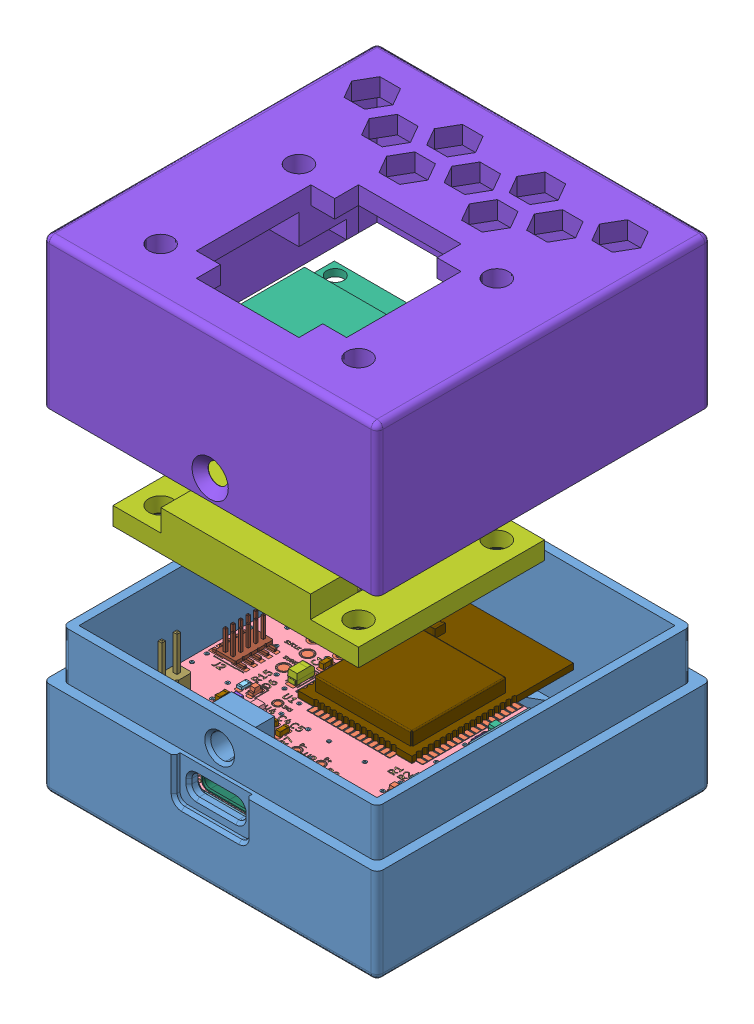
SolidWorks assembly Assem_oled, configuration Default. Lengths in mm.
Overall size (56 81 56).
54 component instances, 26 part files, 31 mates.
Components (placement in the parent):
- case-1: case [Default] at (-21.1368 5.0179 9.443) size (56 24 56)
- UWBkit_minimal-1: UWBkit_minimal [Default] at (-172.7818 2.0179 -67.157) x (1 0 0) z (0 1 0) size (49.01 48.45 15.4)
  - UWBkit_minimal.step-1: UWBkit_minimal.step [Default] at origin size (49.01 48.45 15.4)
    - LED_0603_1608Metric.step-1: LED_0603_1608Metric.step [Default] at (168.7 -85.925 1.595) x (0 -1 0) z (0 0 1) size (1.6 0.8 1.1)
    - SW_PUSH_6mm_H7.3mm.step-1: SW_PUSH_6mm_H7.3mm.step [Default] at (139.45 -64.15 1.595) x (0 -1 0) z (0 0 1) size (7.17 6 10.8)
    - SOT-23-5.step-1: SOT-23-5.step [Default] at (141 -86.775 1.595) x (-1 0 0) z (0 0 1) size (2.8 2.9 1.55)
    - R_0603_1608Metric.step-1: R_0603_1608Metric.step [Default] at (165.5 -82.3 1.595) x (0 1 0) z (0 0 1) size (1.6 0.8 0.45)
    - R_0603_1608Metric.step-2: R_0603_1608Metric.step [Default] at (135.9 -83.2 1.595) x (0 -1 0) z (0 0 1) size (1.6 0.8 0.45)
    - R_0603_1608Metric.step-3: R_0603_1608Metric.step [Default] at (163.9 -82.3 1.595) x (0 1 0) z (0 0 1) size (1.6 0.8 0.45)
    - SOT-23.step-1: SOT-23.step [Default] at (168.1 -68.7 1.595) x (0 1 0) z (0 0 1) size (2.5 3 1.2)
    - CP_EIA-3216-18_Kemet-A.step-1: CP_EIA-3216-18_Kemet-A.step [Default] at (139.6 -77.2775 1.595) x (0 -1 0) z (0 0 1) size (3.2 1.6 1.8)
    - L_0805_2012Metric.step-1: L_0805_2012Metric.step [Default] at (137.8 -86.8 1.595) x (0 1 0) z (0 0 1) size (2 1.25 1.25)
    - C_0603_1608Metric.step-1: C_0603_1608Metric.step [Default] at (139.8 -73.325 1.595) x (0 1 0) z (0 0 1) size (1.6 0.8 0.8)
    - PinSocket_1x02_P2.54mm_Vertical.step-1: PinSocket_1x02_P2.54mm_Vertical.step [Default] at (142.275 -99 1.595) x (0 -1 0) z (0 0 1) size (2.54 5.08 11.6)
    - R_0603_1608Metric.step-4: R_0603_1608Metric.step [Default] at (167.9 -65.8 1.595) x (-1 0 0) z (0 0 1) size (1.6 0.8 0.45)
    - C_0603_1608Metric.step-2: C_0603_1608Metric.step [Default] at (146 -86.8 1.595) x (0 -1 0) z (0 0 1) size (1.6 0.8 0.8)
    - PinHeader_2x05_P1.27mm_Vertical_SMD.step-1: PinHeader_2x05_P1.27mm_Vertical_SMD.step [Default] at (130.8 -78 1.595) x (-1 0 0) z (0 0 1) size (5.57 6.35 4.4)
    - R_0603_1608Metric.step-5: R_0603_1608Metric.step [Default] at (167.8 -75.7 1.595) x (0 1 0) z (0 0 1) size (1.6 0.8 0.45)
    - SOT-23.step-2: SOT-23.step [Default] at (164.5 -68.7 1.595) x (0 1 0) z (0 0 1) size (2.5 3 1.2)
    - PinHeader_1x02_P2.54mm_Vertical.step-1: PinHeader_1x02_P2.54mm_Vertical.step [Default] at (130.8 -89.325 1.595) size (2.54 5.08 11.54)
    - R_0603_1608Metric.step-6: R_0603_1608Metric.step [Default] at (164.8 -75.7 1.595) x (0 1 0) z (0 0 1) size (1.6 0.8 0.45)
    - SOT-23-3.step-1: SOT-23-3.step [Default] at (143.025 -95 1.595) x (0 -1 0) z (0 0 1) size (2.5 3 1.2)
    - PinSocket_1x04_P2.54mm_Vertical.step-1: PinSocket_1x04_P2.54mm_Vertical.step [Default] at (172.7 -79.745 1.595) x (-1 0 0) z (0 0 1) size (2.54 10.16 11.6)
    - R_0603_1608Metric.step-7: R_0603_1608Metric.step [Default] at (164.7 -65.8 1.595) size (1.6 0.8 0.45)
    - LED_0603_1608Metric.step-2: LED_0603_1608Metric.step [Default] at (163.9 -85.925 1.595) x (0 -1 0) z (0 0 1) size (1.6 0.8 1.1)
    - SOT-23.step-3: SOT-23.step [Default] at (139.025 -95 1.595) x (0 -1 0) z (0 0 1) size (2.5 3 1.2)
    - R_0603_1608Metric.step-8: R_0603_1608Metric.step [Default] at (166.3 -75.7 1.595) x (0 1 0) z (0 0 1) size (1.6 0.8 0.45)
    - SOT-23-5.step-2: SOT-23-5.step [Default] at (141.025 -90.6 1.595) x (-1 0 0) z (0 0 1) size (2.8 2.9 1.55)
    - R_0603_1608Metric.step-9: R_0603_1608Metric.step [Default] at (167.9 -64.1 1.595) size (1.6 0.8 0.45)
    - USB_C_Receptacle_GCT_USB4105-xx-A_16P_TopMnt_Horizontal.step-1: USB_C_Receptacle_GCT_USB4105-xx-A_16P_TopMnt_Horizontal.step [Default] at (151.625 -97.94 1.595) size (8.94 7.78 4.26)
    - R_0603_1608Metric.step-10: R_0603_1608Metric.step [Default] at (155.825 -90.6 1.595) x (0 1 0) z (0 0 1) size (1.6 0.8 0.45)
    - C_0603_1608Metric.step-3: C_0603_1608Metric.step [Default] at (144.1 -86.8 1.595) x (0 -1 0) z (0 0 1) size (1.6 0.8 0.8)
    - R_0603_1608Metric.step-11: R_0603_1608Metric.step [Default] at (167.11 -82.3 1.595) x (0 1 0) z (0 0 1) size (1.6 0.8 0.45)
    - C_0603_1608Metric.step-4: C_0603_1608Metric.step [Default] at (135.9 -86.8 1.595) x (0 -1 0) z (0 0 1) size (1.6 0.8 0.8)
    - LED_0603_1608Metric.step-3: LED_0603_1608Metric.step [Default] at (165.5 -85.925 1.595) x (0 -1 0) z (0 0 1) size (1.6 0.8 1.1)
    - LED_0603_1608Metric.step-4: LED_0603_1608Metric.step [Default] at (167.11 -85.925 1.595) x (0 -1 0) z (0 0 1) size (1.6 0.8 1.1)
    - SC-74-6_1.55x2.9mm_P0.95mm.step-1: SC-74-6_1.55x2.9mm_P0.95mm.step [Default] at (151.625 -90.6 1.595) x (-1 0 0) z (0 0 1) size (2.7 2.9 1.18)
    - R_0603_1608Metric.step-12: R_0603_1608Metric.step [Default] at (144.1 -90.6 1.595) x (0 1 0) z (0 0 1) size (1.6 0.8 0.45)
    - LED_0603_1608Metric.step-5: LED_0603_1608Metric.step [Default] at (137.8 -83.2 1.595) x (0 -1 0) z (0 0 1) size (1.6 0.8 1.1)
    - C_0603_1608Metric.step-5: C_0603_1608Metric.step [Default] at (158.325 -99.2 1.595) x (0 -1 0) z (0 0 1) size (1.6 0.8 0.8)
    - R_0603_1608Metric.step-13: R_0603_1608Metric.step [Default] at (164.7 -64.1 1.595) size (1.6 0.8 0.45)
    - R_0603_1608Metric.step-14: R_0603_1608Metric.step [Default] at (158.325 -96.1 1.595) x (0 1 0) z (0 0 1) size (1.6 0.8 0.45)
    - LED_RGB_Wuerth-PLCC4_3.2x2.8mm_150141M173100.step-1: LED_RGB_Wuerth-PLCC4_3.2x2.8mm_150141M173100.step [Default] at (166.3 -72.5 1.595) size (3.5 2.8 2.05)
    - DWM3001C.step-1: DWM3001C.step [Default] at (151.6 -66.71 2.595) size (19.13 27.1 3.2)
    - R_0603_1608Metric.step-15: R_0603_1608Metric.step [Default] at (168.7 -82.3 1.595) x (0 1 0) z (0 0 1) size (1.6 0.8 0.45)
    - R_0603_1608Metric.step-16: R_0603_1608Metric.step [Default] at (147.325 -90.6 1.595) x (0 1 0) z (0 0 1) size (1.6 0.8 0.45)
    - BatteryHolder_Keystone_1058_1x2032.step-1: BatteryHolder_Keystone_1058_1x2032.step [Default] at (151.625 -82.7 -0.085) x (1 0 0) z (0 0 -1) size (31.86 16 5.08)
    - UWBkit_minimal_pad.step-1: UWBkit_minimal_pad.step [Default] at origin size (47.72 38.11 1.59)
    - UWBkit_minimal_silkscreen.step-1: UWBkit_minimal_silkscreen.step [Default] at origin size (46.73 38.02 1.67)
    - UWBkit_minimal_soldermask.step-1: UWBkit_minimal_soldermask.step [Default] at origin size (49.01 39.11 1.62)
    - UWBkit_minimal_PCB.step-1: UWBkit_minimal_PCB.step [Default] at origin size (49 39.1 1.51)
- oled-1: oled [Default] at (-21.1868 59.8179 17.543) size (25 2.8 27)
- oled_holder-1: oled_holder [Default] at (-21.1368 33.0179 17.543) size (41.2 6.7 31.2)
- lid_oled-1: lid_oled [Default] at (-21.1368 74.0179 9.443) x (-1 0 0) z (0 0 1) size (56 25 56)
Mates (geometry in assembly coordinates):
- Coincident1: coincident anti-aligned: plane of case-1 through (-21.1368 2.0179 9.443) normal (0 1 0); plane of UWBkit_minimal.step-1/UWBkit_minimal_PCB.step-1 through (-172.7618 2.0179 -67.157) normal (0 -1 0)
- Distance1: distance = 0.5 mm anti-aligned: plane of UWBkit_minimal.step-1/UWBkit_minimal_PCB.step-1 through (-45.6368 2.0179 33.443) normal (-1 0 0); plane of case-1 through (-46.1368 14.0179 34.443) normal (1 0 0)
- Coincident3: coincident anti-aligned: plane of case-1 through (-46.1368 14.0179 34.443) normal (0 0 -1); plane of UWBkit_minimal.step-1/UWBkit_minimal_PCB.step-1 through (2.3632 2.0179 34.443) normal (0 0 1)
- Coincident7: coincident: plane of case-1 through (-46.1368 14.0179 34.443) normal (0 0 -1); plane of UWBkit_minimal.step-2/UWBkit_minimal_PCB.step-1 through (2.3632 2.0179 34.443) normal (0 0 1)
- Distance2: distance = 0.5 mm: plane of UWBkit_minimal.step-2/UWBkit_minimal_PCB.step-1 through (-45.6368 2.0179 33.443) normal (-1 0 0); plane of case-1 through (-46.1368 14.0179 34.443) normal (1 0 0)
- Coincident9: coincident anti-aligned: plane of case-1 through (-21.1368 2.0179 9.443) normal (0 1 0); plane of UWBkit_minimal.step-2/UWBkit_minimal_PCB.step-1 through (-172.7618 2.0179 -67.157) normal (0 -1 0)
- Coincident10: coincident anti-aligned: plane of case-1 through (-21.1368 2.0179 9.443) normal (0 1 0); plane of UWBkit_minimal-1/UWBkit_minimal.step-1/UWBkit_minimal_PCB.step-1 through (-172.7818 2.0179 -67.157) normal (0 -1 0)
- Concentric1: concentric anti-aligned: cylinder of case-1 through (-0.1568 -12.639 -1.157) axis (0 1 0) radius 2; cylinder of UWBkit_minimal-1/UWBkit_minimal.step-1/UWBkit_minimal_pad.step-1 through (-0.1568 1.9719 -1.157) axis (0 -1 0) radius 1.575
- Parallel1: parallel anti-aligned: plane of case-1 through (-46.1368 14.0179 34.443) normal (0 0 -1); plane of UWBkit_minimal-1/UWBkit_minimal.step-1/UWBkit_minimal_PCB.step-1 through (2.3432 2.0179 34.443) normal (0 0 1)
- Parallel2: parallel aligned: line of case-1 through (4.2632 9.0179 -16.957) axis (-1 0 0); line of oled-1 through (-8.6868 59.8179 4.043) axis (-1 0 0)
- Distance5: distance = 5 mm anti-aligned: plane of oled-1 through (-33.6868 61.0179 31.043) normal (0 0 1); plane of lid_oled-1 through (5.4632 71.0179 36.043) normal (0 0 -1)
- Distance6: distance = 0 mm aligned: plane of lid-1 through (-49.1368 9.0179 37.443) normal (-1 0 0); plane of case-1 through (-49.1368 14.0179 34.443) normal (-1 0 0)
- Distance7: distance = 0 mm aligned: plane of lid-1 through (6.8632 9.0179 37.443) normal (0 0 1); plane of case-1 through (-46.1368 14.0179 37.443) normal (0 0 1)
- LimitDistance1: limit distance = 0 mm anti-aligned: plane of lid-1 through (-21.1368 9.0179 9.443) normal (0 -1 0); plane of case-1 through (-21.1368 9.0179 9.443) normal (0 1 0)
- Distance10: distance = 0 mm aligned: plane of lid-1 through (-41.7368 26.0179 25.143) normal (-1 0 0); plane of oled_holder-1 through (-41.7368 26.0179 33.143) normal (-1 0 0)
- LimitDistance2: limit distance = 0 mm anti-aligned: plane of lid-1 through (-21.1368 26.0179 9.443) normal (0 -1 0); plane of oled_holder-1 through (-21.1368 26.0179 17.543) normal (0 1 0)
- Coincident24: coincident anti-aligned: plane of lid-1 through (-21.1368 26.0179 9.443) normal (0 -1 0); plane of oled_holder_part-2 through (-6.5368 76.0179 5.943) normal (0 1 0)
- Coincident25: coincident anti-aligned: plane of lid-1 through (-0.5368 23.0179 1.943) normal (-1 0 0); plane of oled_holder_part-2 through (-0.5368 76.0179 9.943) normal (1 0 0)
- Coincident26: coincident anti-aligned: plane of lid-1 through (-8.5368 23.0179 1.943) normal (0 0 1); plane of oled_holder_part-2 through (-12.5368 76.0179 1.943) normal (0 0 -1)
- Coincident27: coincident anti-aligned: plane of lid-1 through (-21.1368 26.0179 9.443) normal (0 -1 0); plane of oled_holder_part-1 through (-35.7368 76.0179 5.943) normal (0 1 0)
- Coincident29: coincident anti-aligned: plane of lid-1 through (-41.7368 23.0179 1.943) normal (1 0 0); plane of oled_holder_part-1 through (-41.7368 76.0179 1.943) normal (-1 0 0)
- Coincident30: coincident anti-aligned: plane of lid-1 through (-33.7368 23.0179 1.943) normal (0 0 1); plane of oled_holder_part-1 through (-29.7368 76.0179 1.943) normal (0 0 -1)
- Distance13: distance = 0 mm aligned: plane of lid-1 through (-41.7368 26.0179 33.143) normal (0 0 1); plane of oled_holder-1 through (-41.7368 26.0179 33.143) normal (0 0 1)
- Distance14: distance = 0 mm aligned: plane of lid_oled-1 through (6.8632 49.0179 37.443) normal (0 0 1); plane of case-1 through (-46.1368 14.0179 37.443) normal (0 0 1)
- Distance16: distance = 0 mm aligned: plane of lid_oled-1 through (6.8632 49.0179 37.443) normal (1 0 0); plane of case-1 through (6.8632 14.0179 34.443) normal (1 0 0)
- LimitDistance4: limit distance = 40 mm anti-aligned: plane of lid_oled-1 through (-21.1368 49.0179 9.443) normal (0 -1 0); plane of case-1 through (-21.1368 9.0179 9.443) normal (0 1 0)
- Distance18: distance = 0.05 mm anti-aligned: plane of oled-1 through (-33.6868 61.0179 31.043) normal (-1 0 0); plane of lid_oled-1 through (-33.7368 33.9385 31.143) normal (1 0 0)
- LimitDistance5: limit distance = 10 mm anti-aligned: plane of oled-1 through (-21.1868 61.0179 17.543) normal (0 1 0); plane of lid_oled-1 through (-21.1368 71.0179 9.443) normal (0 -1 0)
- Distance21: distance = 0 mm aligned: plane of oled_holder-1 through (-41.7368 36.0179 33.143) normal (0 0 1); plane of lid_oled-1 through (-8.5368 66.0179 33.143) normal (0 0 1)
- Distance22: distance = 0 mm aligned: plane of oled_holder-1 through (-41.7368 36.0179 33.143) normal (-1 0 0); plane of lid_oled-1 through (-41.7368 66.0179 25.143) normal (-1 0 0)
- LimitDistance6: limit distance = 30 mm anti-aligned: plane of oled_holder-1 through (-21.1368 36.0179 17.543) normal (0 1 0); plane of lid_oled-1 through (-21.1368 66.0179 9.443) normal (0 -1 0)
